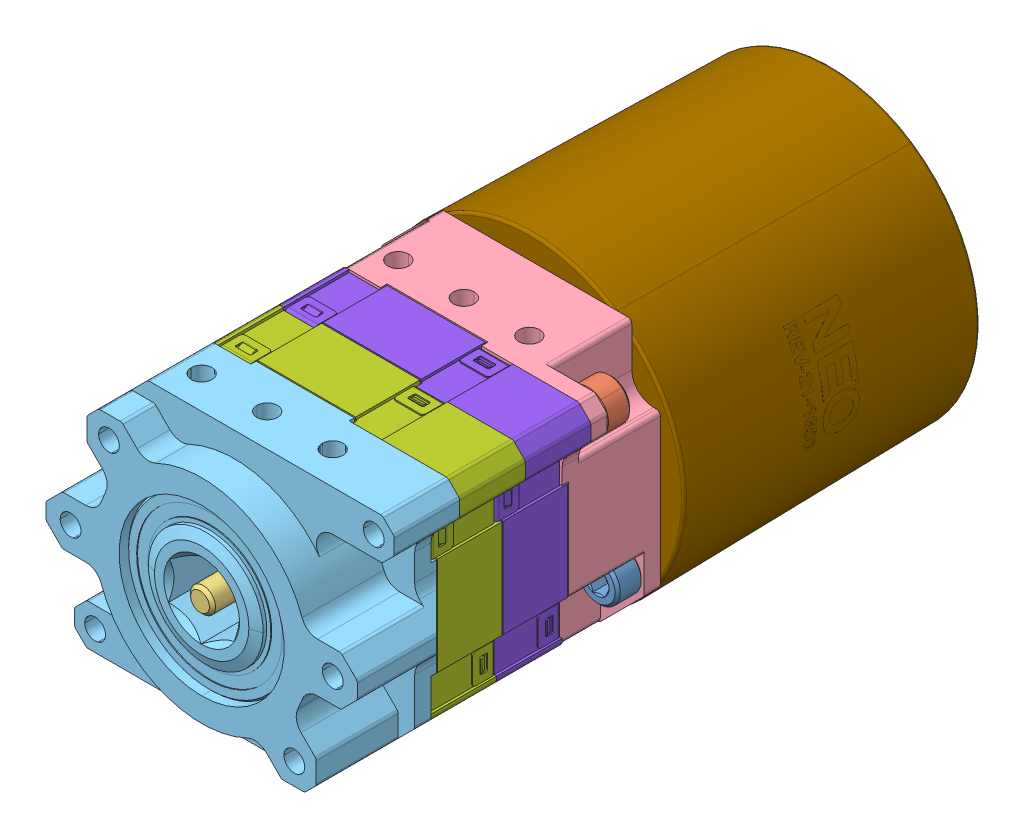
SolidWorks assembly MAXPlanetary 2-Stage, configuration Default. Lengths in mm.
Overall size (89.61 89.51 122.08).
14 component instances, 9 part files, 0 mates.
Components (placement in the parent):
- MAXPlanetary 2-Stage.STEP-1: MAXPlanetary 2-Stage.STEP [Default] at origin size (89.61 89.51 122.08)
  - REV-25-2109_2-Stage (No Shaft, For NEO).STEP-1: REV-25-2109_2-Stage (No Shaft, For NEO).STEP [Default] at origin size (65.15 54.03 73.34)
    - REV-25-2107_2-Stage.STEP-1: REV-25-2107_2-Stage.STEP [Default] at (0 0 6.35) x (-1 0 0) z (0 0 -1) size (65.15 54.03 73.34)
      - #10 Socket Head Cap Screws_0.500in Long.STEP-1: #10 Socket Head Cap Screws_0.500in Long.STEP [Default] at (21.1355 14.0872 12.7) x (0.923728 0.383049 0) z (0.383049 -0.923728 0) size (7.94 17.53 7.94)
      - #10 Socket Head Cap Screws_0.500in Long.STEP-2: #10 Socket Head Cap Screws_0.500in Long.STEP [Default] at (-21.1355 -14.0872 12.7) x (0.923728 0.383049 0) z (0.383049 -0.923728 0) size (7.94 17.53 7.94)
      - #10 Socket Head Cap Screws_1.500in Long.STEP-1: #10 Socket Head Cap Screws_1.500in Long.STEP [Default] at (-26.9919 21.4312 0) x (0.777574 0.628792 0) z (-0.628792 0.777574 0) size (7.94 42.93 7.94)
      - #10 Socket Head Cap Screws_1.500in Long.STEP-2: #10 Socket Head Cap Screws_1.500in Long.STEP [Default] at (26.9919 -21.4312 0) x (0.777574 0.628792 0) z (-0.628792 0.777574 0) size (7.94 42.93 7.94)
      - #10-32 Button Head Cap Screws_0.500in Long.STEP-1: #10-32 Button Head Cap Screws_0.500in Long.STEP [Default] at (0 0 -35.2425) x (0.655967 -0.754789 0) z (-0.754789 -0.655967 0) size (9.17 15.27 9.17)
    - REV-21-2106.STEP-1: REV-21-2106.STEP [Default] at origin size (61.91 50.8 19.05)
    - REV-21-2104.STEP-1: REV-21-2104.STEP [Default] at (0 0 44.45) x (0 0 1) z (-1 0 0) size (23.2 50.8 61.92)
    - REV-21-2108.STEP-1: REV-21-2108.STEP [Default] at (0 0 7.0985) x (-0.554615 -0.832107 0) z (0 0 -1) size (25.4 25.4 14.94)
  - REV-21-2101.STEP-1: REV-21-2101.STEP [Default] at (0 0 28.575) size (61.91 50.8 16.85)
  - REV-21-2102.STEP-1: REV-21-2102.STEP [Default] at (0 0 15.875) size (61.91 50.8 16.85)
  - REV-21-1650.STEP-1: REV-21-1650.STEP [Default] at (0 0 -9.525) x (0.554615 0.832107 0) z (0 0 1) size (64.41 64.76 93.26)
